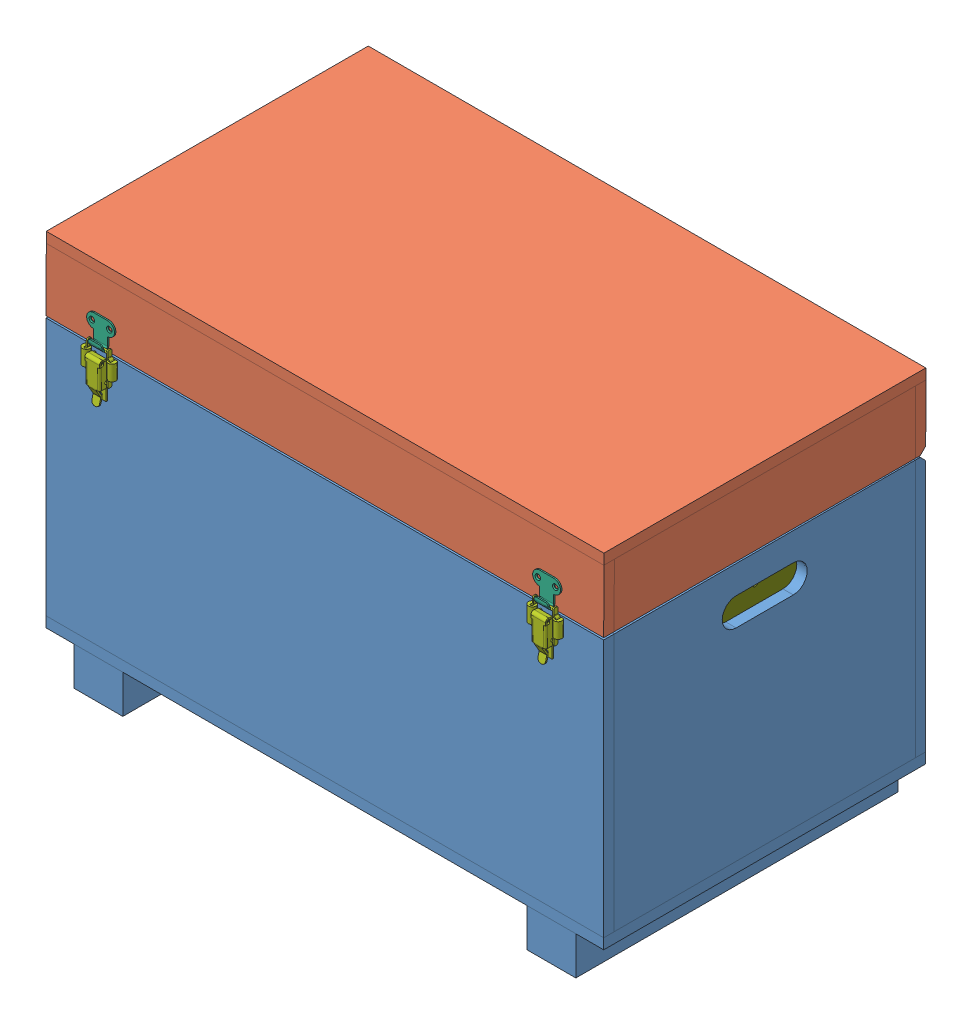
SolidWorks assembly 2021_CaisseTransport, configuration Default. Lengths in mm.
Overall size (800 575.29 476.19).
36 component instances, 27 part files, 81 mates.
Components (placement in the parent):
- 2021_Caisse_Fond-1: 2021_Caisse_Fond [Default] at origin size (800 446 462)
- 2021_Caisse_Capot-1: 2021_Caisse_Capot [Default] at (0 492.3908 -0.1871) x (-1 0 0) z (0 0.001745 0.999998) size (800 124 462)
- _2021_RobotPrincipal_FacesExt-1: _2021_RobotPrincipal_FacesExt [Default] at (-195 34.5 15) x (0 0 -1) z (1 0 0) size (333 431 295.5)
- _2021_RobotSecondaire_FacesExt-1: _2021_RobotSecondaire_FacesExt [Default] at (72 34.5 -65) x (-1 0 0) z (0 0 -1) size (273 428.5 191)
- _2021_Phare_FacesExt-1: _2021_Phare_FacesExt [Default] at (146 145 117) x (-1 0 0) z (0 0 -1) size (440.05 342.73 212.15)
- carton_clavier_logitech_k400-1: carton_clavier_logitech_k400 [Défaut] at (-278.5 201 -214) x (0 -1 0) z (-1 0 0) size (372 32 155)
- Plateau roulant Manutention-1: Plateau roulant Manutention [Défaut] x (-1 0 0) z (0 0 -1) size (575 82.5 290)
- StationAccueil-1: StationAccueil [Défaut] at (17 215 -192) x (0 1 0) z (1 0 0) size (428 34 400)
- GL-210606-0849_CaissePce01-1: GL-210606-0849_CaissePce01 [Default] at (-192 215 -216) size (43.02 40.06 45)
- GL-210606-0853_CaissePce02-1: GL-210606-0853_CaissePce02 [Default] at (-364 210 -216) size (26.02 40.06 45)
- GL-210606-0904_CaissePce03-1: GL-210606-0904_CaissePce03 [Default] at (217 210 -151) x (-1 0 0) z (0 0 -1) size (16.03 40.06 30)
- GL-210606-0912_CaissePce04-1: GL-210606-0912_CaissePce04 [Default] at (-385 374 147) size (10.79 44 25.48)
- GL-210606-0912_CaissePce04-2: GL-210606-0912_CaissePce04 [Default] at (385 374 147) x (-1 0 0) z (0 0 -1) size (10.79 44 25.48)
- GL-210606-0912_CaissePce04-3: GL-210606-0912_CaissePce04 [Default] at (-78 134 189) x (-1 0 0) z (0 0 -1) size (10.79 44 25.48)
- GL-210606-0943_CaissePce05-1: GL-210606-0943_CaissePce05 [Default] at (-56.5 15 -118.5) size (45.57 49.43 53.44)
- GL-210606-0943_CaissePce05-2: GL-210606-0943_CaissePce05 [Default] at (200.5 15 -11.5) x (-1 0 0) z (0 0 -1) size (45.57 49.43 53.44)
- GL-210606-0943_CaissePce05_Sym-3: GL-210606-0943_CaissePce05_Sym [Default] at (-56.5 15 -11.5) size (45.57 49.43 53.44)
- GL-210606-0943_CaissePce05_Sym-4: GL-210606-0943_CaissePce05_Sym [Default] at (200.5 15 -118.5) x (-1 0 0) z (0 0 -1) size (45.57 49.43 53.44)
- GL-210606-1029_CaissePce06-1: GL-210606-1029_CaissePce06 [Default] at (-141.5 15 -143.5) x (0 0 1) z (-1 0 0) size (35.58 49.93 35.5)
- _2021_VisionCentrale_FacesExt-1: _2021_VisionCentrale_FacesExt [Default] at (275.4 230 -111) x (0 1 0) z (0 0 1) size (244.44 54.3 190)
- GL-210606-1436_CaissePce07-2: GL-210606-1436_CaissePce07 [Default] at (-248.5 15 173.5) x (0 0 -1) z (1 0 0) size (35.58 49.43 55.65)
- GL-210606-1436_CaissePce07_Sym-2: GL-210606-1436_CaissePce07_Sym [Default] at (-248.5 15 -143.5) x (0 0 1) z (-1 0 0) size (35.58 49.43 55.65)
- GL-210606-1029_CaissePce06_Sym-2: GL-210606-1029_CaissePce06_Sym [Default] at (-141.5 15 173.5) x (0 0 -1) z (1 0 0) size (35.58 49.93 35.5)
- GL-210606-1457_CaissePce08-1: GL-210606-1457_CaissePce08 [Default] at (-346 15 15) size (27.07 49.43 30)
- GL-210606-1507_CaissePce09-2: GL-210606-1507_CaissePce09 [Default] at (235 132 -7) x (0 0 -1) z (1 0 0) size (32 160 63.05)
- GL-210606-1507_CaissePce09_Sym-3: GL-210606-1507_CaissePce09_Sym [Default] at (235 132 -215) x (0 0 1) z (-1 0 0) size (32 160 63.05)
- GL-210606-1534_CaissePce10-1: GL-210606-1534_CaissePce10 [Default] at (-342.5 330 216) x (0 0 -1) z (0 -1 0) size (30.57 15 56.89)
- GL-210606-1534_CaissePce10-2: GL-210606-1534_CaissePce10 [Default] at (-297.5 330 216) x (0 0 -1) z (0 -1 0) size (30.57 15 56.89)
- FermoirRessort_PartB-1: FermoirRessort_PartB [Default] at (-320 417.7941 230.9435) x (1 0 0) z (0 0.001745 0.999998) size (40 37 10)
- FermoirRessort_PartA-1: FermoirRessort_PartA [Default] at (-320 360 231) size (48 75.52 15.5)
- FermoirRessort_PartA-2: FermoirRessort_PartA [Default] at (320 360 231) size (48 75.52 15.5)
- FermoirRessort_PartB-2: FermoirRessort_PartB [Default] at (320 417.7941 230.9435) x (1 0 0) z (0 0.001745 0.999998) size (40 37 10)
- GL-210607-2320_CaissePce11-1: GL-210607-2320_CaissePce11 [Default] at (-195 470.6875 169.851) x (1 0 0) z (0 -0.001745 -0.999998) size (190 80 29)
- GL-210607-2320_CaissePce11-2: GL-210607-2320_CaissePce11 [Default] at (-195 470.1465 -140.1485) x (1 0 0) z (0 -0.001745 -0.999998) size (190 80 29)
- GL-210607-2322_CaissePce12-1: GL-210607-2322_CaissePce12 [Default] at (-53 470.2774 -65.1486) x (0 0.001745 0.999998) z (1 0 0) size (220 80 29)
- GL-210607-2322_CaissePce12-2: GL-210607-2322_CaissePce12 [Default] at (197 470.2774 -65.1486) x (0 0.001745 0.999998) z (1 0 0) size (220 80 29)
Mates (geometry in assembly coordinates):
- Coïncidente1: coincident: circle of assembly; circle of assembly; circle of 2021_Caisse_Fond-1; circle of 2021_Caisse_Capot-1
- AngleLimite1: limit planar angle = 0.001745 rad: plane of assembly; plane of assembly; plane of 2021_Caisse_Capot-1 through (0 387.391 -0.0038) normal (0 -0.999998 0.001745); plane of 2021_Caisse_Fond-1 through (0 385 0) normal (0 1 0)
- Distance12: distance = 25 mm: plane of assembly; plane of assembly; plane of _2021_RobotSecondaire_FacesExt-1 through (72 40 -105) normal (0 -1 0); plane of 2021_Caisse_Fond-1 through (0 15 0) normal (0 1 0)
- Distance13: distance = 25 mm: plane of _2021_RobotPrincipal_FacesExt-1 through (-195 40 15) normal (0 -1 0); plane of 2021_Caisse_Fond-1 through (0 15 0) normal (0 1 0)
- Coïncidente26: coincident: plane of assembly; plane of assembly; plane of 2021_Caisse_Fond-1 through (0 15 0) normal (0 1 0); plane of StationAccueil-1 through (217 15 -214) normal (0 -1 0)
- Coïncidente13: coincident: plane of assembly; plane of assembly; plane of 2021_Caisse_Fond-1 through (0 0 0) normal (0 -1 0); plane of Plateau roulant Manutention-1 through (0 0 0) normal (0 1 0)
- Coïncidente14: coincident: plane of assembly through (0 0 0) normal (0 0 1); plane of Plateau roulant Manutention-1 through (0 0 0) normal (0 0 -1); plane of assembly
- Coïncidente15: coincident: plane of assembly through (0 0 0) normal (1 0 0); plane of Plateau roulant Manutention-1 through (0 0 0) normal (-1 0 0); plane of assembly
- Distance19: distance = 72 mm: plane of assembly through (0 0 0) normal (1 0 0); plane of assembly; plane of _2021_RobotSecondaire_FacesExt-1 through (72 34.5 -65) normal (-1 0 0)
- Distance6: distance = 65 mm: plane of assembly through (0 0 0) normal (0 0 1); plane of _2021_RobotSecondaire_FacesExt-1 through (72 34.5 -65) normal (0 0 -1); plane of assembly
- Distance7: distance = 195 mm: plane of _2021_RobotPrincipal_FacesExt-1 through (-195 34.5 15) normal (1 0 0); plane of assembly through (0 0 0) normal (1 0 0)
- Distance14: distance = 15 mm: plane of _2021_RobotPrincipal_FacesExt-1 through (-195 34.5 15) normal (0 0 -1); plane of assembly through (0 0 0) normal (0 0 1)
- Distance11: distance = 130 mm: plane of assembly; plane of assembly; plane of _2021_Phare_FacesExt-1 through (146 145 117) normal (0 -1 0); plane of 2021_Caisse_Fond-1 through (0 15 0) normal (0 1 0)
- Distance15: distance = 1 mm: plane of StationAccueil-1 through (17 215 -215) normal (0 0 -1); plane of 2021_Caisse_Fond-1 through (-400 385 -216) normal (0 0 1)
- Distance16: distance = 2 mm: plane of assembly; plane of assembly; plane of carton_clavier_logitech_k400-1 through (-278.5 201 -214) normal (0 0 -1); plane of 2021_Caisse_Fond-1 through (-400 385 -216) normal (0 0 1)
- Coïncidente29: coincident: plane of 2021_Caisse_Fond-1 through (0 15 0) normal (0 1 0); plane of carton_clavier_logitech_k400-1 through (-356 15 -182) normal (0 -1 0)
- Distance17: distance = 4 mm: plane of _2021_Phare_FacesExt-1 through (366 373.5 145) normal (1 0 0); plane of 2021_Caisse_Fond-1 through (370 434.3356 216) normal (-1 0 0)
- Distance18: distance = 4 mm: plane of _2021_Phare_FacesExt-1 through (366 146.5 212) normal (0 0 1); plane of 2021_Caisse_Fond-1 through (-400 385 216) normal (0 0 -1)
- Distance20: distance = 3 mm: plane of StationAccueil-1 through (217 415 -214) normal (1 0 0); plane of 2021_Caisse_Fond-1 through (220 527.429 -216) normal (-1 0 0)
- Distance21: distance = 18 mm: plane of StationAccueil-1 through (-183 15 -214) normal (-1 0 0); plane of carton_clavier_logitech_k400-1 through (-201 387 -182) normal (1 0 0)
- Coïncidente30: coincident: plane of assembly; plane of assembly; plane of 2021_Caisse_Fond-1 through (-400 385 -216) normal (0 0 1); plane of GL-210606-0849_CaissePce01-1 through (-199.5 235 -216) normal (0 0 -1)
- Distance22: distance = 9 mm: plane of GL-210606-0849_CaissePce01-1 through (-192 215 -216) normal (1 0 0); plane of StationAccueil-1 through (-183 15 -214) normal (-1 0 0)
- Distance23: distance = 220 mm: plane of GL-210606-0849_CaissePce01-1 through (-192 235 -216) normal (0 1 0); plane of 2021_Caisse_Fond-1 through (0 15 0) normal (0 1 0)
- Coïncidente33: coincident: plane of GL-210606-0849_CaissePce01-1 through (-192 235 -216) normal (0 1 0); plane of GL-210606-0853_CaissePce02-1 through (-364 235 -216) normal (0 1 0)
- Coïncidente34: coincident: plane of 2021_Caisse_Fond-1 through (-370 434.3356 -216) normal (1 0 0); plane of GL-210606-0853_CaissePce02-1 through (-370 195 -171) normal (-1 0 0)
- Coïncidente35: coincident: plane of 2021_Caisse_Fond-1 through (-400 385 -216) normal (0 0 1); plane of GL-210606-0853_CaissePce02-1 through (-370 195 -216) normal (0 0 -1)
- Coïncidente36: coincident: plane of GL-210606-0849_CaissePce01-1 through (-192 235 -216) normal (0 1 0); plane of GL-210606-0904_CaissePce03-1 through (217 235 -151) normal (0 1 0)
- Coïncidente37: coincident: plane of GL-210606-0849_CaissePce01-1 through (-184.5 235 -181) normal (0 0 -1); plane of GL-210606-0904_CaissePce03-1 through (204 195 -181) normal (0 0 -1)
- Coïncidente38: coincident: plane of 2021_Caisse_Fond-1 through (220 527.429 -216) normal (-1 0 0); plane of GL-210606-0904_CaissePce03-1 through (220 195 -181) normal (1 0 0)
- Distance28: distance = 15 mm: plane of assembly; plane of assembly; plane of 2021_Caisse_Fond-1 through (-400 385 216) normal (0 0 -1); plane of GL-210606-0912_CaissePce04-3 through (-78 120 201) normal (0 0 1)
- Coïncidente40: coincident: plane of 2021_Caisse_Fond-1 through (-78 145 216) normal (-1 0 0); plane of GL-210606-0912_CaissePce04-3 through (-78 120 177) normal (1 0 0)
- Coïncidente41: coincident: plane of assembly; plane of assembly; plane of GL-210606-0912_CaissePce04-1 through (-375 360 159) normal (0 0 1); plane of GL-210606-0912_CaissePce04-2 through (385 360 159) normal (0 0 1)
- Coïncidente42: coincident: plane of GL-210606-0912_CaissePce04-1 through (-385 404 147) normal (0 1 0); plane of GL-210606-0912_CaissePce04-2 through (385 404 147) normal (0 1 0)
- Coïncidente43: coincident: plane of 2021_Caisse_Fond-1 through (-385 385 -216) normal (1 0 0); plane of GL-210606-0912_CaissePce04-1 through (-385 360 159) normal (-1 0 0)
- Coïncidente44: coincident: plane of 2021_Caisse_Fond-1 through (385 385 -216) normal (-1 0 0); plane of GL-210606-0912_CaissePce04-2 through (385 360 135) normal (1 0 0)
- Distance24: distance = 10 mm: plane of GL-210606-0912_CaissePce04-2 through (385 360 159) normal (0 0 1); plane of 2021_Caisse_Fond-1 through (385 434.3356 169) normal (0 0 -1)
- Distance26: distance = 25 mm: plane of GL-210606-0912_CaissePce04-1 through (-385 360 147) normal (0 -1 0); plane of 2021_Caisse_Fond-1 through (0 385 0) normal (0 1 0)
- Distance27: distance = 25 mm: plane of GL-210606-0912_CaissePce04-3 through (-78 120 189) normal (0 -1 0); plane of 2021_Caisse_Fond-1 through (0 145 0) normal (0 1 0)
- Coïncidente49: coincident: plane of assembly; plane of assembly; plane of 2021_Caisse_Fond-1 through (0 15 0) normal (0 1 0); plane of GL-210606-0943_CaissePce05-1 through (-56.5 15 -118.5) normal (0 -1 0)
- Coaxiale1: concentric: point of assembly; cylinder of assembly; point of GL-210606-0943_CaissePce05-1; cylinder of _2021_RobotSecondaire_FacesExt-1 through (-56.5 50.25 -118.5) axis (0 -1 0) radius 8
- Parallèle2: parallel: plane of assembly; plane of assembly; plane of _2021_RobotSecondaire_FacesExt-1 through (72 45.5 -5) normal (0 0 1); plane of GL-210606-0943_CaissePce05-1 through (-56.5 15 -118.5) normal (0 0 1)
- Coïncidente53: coincident: plane of assembly; plane of assembly; plane of GL-210606-0943_CaissePce05-1 through (-56.5 15 -118.5) normal (0 -1 0); plane of GL-210606-0943_CaissePce05-2 through (200.5 15 -11.5) normal (0 -1 0)
- Parallèle3: parallel: plane of assembly; plane of assembly; plane of GL-210606-0943_CaissePce05-1 through (-64 40 -102.5) normal (0 0 1); plane of GL-210606-0943_CaissePce05-2 through (208 40 -27.5) normal (0 0 -1)
- Coaxiale2: concentric: cylinder of assembly; point of assembly; cylinder of _2021_RobotSecondaire_FacesExt-1 through (200.5 50.25 -11.5) axis (0 -1 0) radius 8; point of GL-210606-0943_CaissePce05-2
- Coïncidente56: coincident: plane of 2021_Caisse_Fond-1 through (0 15 0) normal (0 1 0); plane of GL-210606-1029_CaissePce06-1 through (-141.5 15 -143.5) normal (0 -1 0)
- Coaxiale3: concentric: cylinder of _2021_RobotPrincipal_FacesExt-1 through (-141.5 50.25 -143.5) axis (0 -1 0) radius 8; unknown of GL-210606-1029_CaissePce06-1
- Parallèle4: parallel: plane of _2021_RobotPrincipal_FacesExt-1 through (-135 45.5 15) normal (1 0 0); plane of GL-210606-1029_CaissePce06-1 through (-141.5 15 -143.5) normal (-1 0 0)
- Distance29: distance = 8 mm: plane of _2021_VisionCentrale_FacesExt-1 through (243 315 -206) normal (-1 0 0); plane of 2021_Caisse_Fond-1 through (235 527.429 -216) normal (1 0 0)
- Distance30: distance = 10 mm: plane of _2021_VisionCentrale_FacesExt-1 through (247.1 135 -206) normal (0 0 -1); plane of 2021_Caisse_Fond-1 through (-400 385 -216) normal (0 0 1)
- Distance31: distance = 120 mm: plane of _2021_VisionCentrale_FacesExt-1 through (247.1 135 -206) normal (0 -1 0); plane of 2021_Caisse_Fond-1 through (0 15 0) normal (0 1 0)
- Coïncidente57: coincident: plane of 2021_Caisse_Fond-1 through (0 15 0) normal (0 1 0); plane of GL-210606-1436_CaissePce07-2 through (-195 15 15) normal (0 -1 0)
- Coaxiale4: concentric: cylinder of _2021_RobotPrincipal_FacesExt-1 through (-248.5 50.25 173.5) axis (0 -1 0) radius 8; unknown of GL-210606-1436_CaissePce07-2
- Parallèle5: parallel: plane of _2021_RobotPrincipal_FacesExt-1 through (-255 45.5 180) normal (0 0 1); plane of GL-210606-1436_CaissePce07-2 through (-248.5 15 173.5) normal (0 0 -1)
- Coïncidente60: coincident: plane of assembly; plane of assembly; plane of 2021_Caisse_Fond-1 through (0 15 0) normal (0 1 0); plane of GL-210606-1457_CaissePce08-1 through (-346 15 15) normal (0 -1 0)
- Distance32: distance = 1 mm: plane of GL-210606-1457_CaissePce08-1 through (-346 -17.311 0) normal (1 0 0); plane of _2021_RobotPrincipal_FacesExt-1 through (-345 41.5 -73.1816) normal (-1 0 0)
- Coïncidente62: coincident: plane of _2021_RobotPrincipal_FacesExt-1 through (-195 34.5 15) normal (0 0 -1); plane of GL-210606-1457_CaissePce08-1 through (-346 15 15) normal (0 0 1)
- Coïncidente63: coincident: plane of 2021_Caisse_Fond-1 through (235 527.429 -216) normal (1 0 0); plane of GL-210606-1507_CaissePce09-2 through (235 292 -26) normal (-1 0 0)
- Coïncidente64: coincident: plane of 2021_Caisse_Fond-1 through (0 265 0) normal (0 1 0); plane of GL-210606-1507_CaissePce09-2 through (235 265 -22) normal (0 -1 0)
- Distance33: distance = 2 mm: plane of GL-210606-1507_CaissePce09-2 through (242 292 -14) normal (0 0 -1); plane of _2021_VisionCentrale_FacesExt-1 through (247.1 135 -16) normal (0 0 1)
- Coïncidente66: coincident: plane of assembly; plane of assembly; plane of 2021_Caisse_Fond-1 through (-400 385 216) normal (0 0 -1); plane of GL-210606-1534_CaissePce10-1 through (-335 350 216) normal (0 0 1)
- Distance34: distance = 20 mm: plane of GL-210606-1534_CaissePce10-1 through (-350 352.8914 203.4271) normal (-1 0 0); plane of 2021_Caisse_Fond-1 through (-370 434.3356 216) normal (1 0 0)
- Distance35: distance = 35 mm: plane of GL-210606-1534_CaissePce10-1 through (-335 350 213) normal (0 1 0); plane of 2021_Caisse_Fond-1 through (0 385 0) normal (0 1 0)
- Coïncidente69: coincident: plane of GL-210606-1534_CaissePce10-1 through (-335 350 216) normal (0 0 1); plane of GL-210606-1534_CaissePce10-2 through (-290 350 216) normal (0 0 1)
- Coïncidente70: coincident: plane of GL-210606-1534_CaissePce10-1 through (-335 350 213) normal (0 1 0); plane of GL-210606-1534_CaissePce10-2 through (-290 350 213) normal (0 1 0)
- Distance36: distance = 30 mm: plane of GL-210606-1534_CaissePce10-1 through (-335 352.8914 203.4271) normal (1 0 0); plane of GL-210606-1534_CaissePce10-2 through (-305 352.8914 203.4271) normal (-1 0 0)
- Coïncidente72: coincident: plane of assembly; plane of assembly; plane of 2021_Caisse_Capot-1 through (400 387.7941 230.9958) normal (0 0.001745 0.999998); plane of FermoirRessort_PartB-1 through (-310 427.7941 230.926) normal (0 -0.001745 -0.999998)
- Distance37: distance = 80 mm: plane of assembly; plane of assembly; plane of FermoirRessort_PartB-1 through (-320 417.7941 230.9435) normal (1 0 0); plane of 2021_Caisse_Capot-1 through (-400 387.014 -216.0035) normal (-1 0 0)
- Distance38: distance = 30 mm: plane of assembly; plane of assembly; plane of FermoirRessort_PartB-1 through (-320 417.7941 230.9435) normal (0 0.999998 -0.001745); plane of 2021_Caisse_Capot-1 through (0 387.391 -0.0038) normal (0 -0.999998 0.001745)
- Coïncidente75: coincident: plane of assembly; plane of assembly; plane of 2021_Caisse_Fond-1 through (-400 385 231) normal (0 0 1); plane of FermoirRessort_PartA-1 through (-312 326 231) normal (0 0 -1)
- Coïncidente76: coincident: plane of assembly; plane of assembly; plane of FermoirRessort_PartB-1 through (-320 417.7941 230.9435) normal (1 0 0); plane of FermoirRessort_PartA-1 through (-320 360 231) normal (1 0 0)
- Distance39: distance = 25 mm: plane of assembly; plane of assembly; plane of FermoirRessort_PartA-1 through (-320 360 231) normal (0 1 0); plane of 2021_Caisse_Fond-1 through (0 385 0) normal (0 1 0)
- Coïncidente77: coincident: plane of assembly; plane of assembly; plane of GL-210607-2322_CaissePce12-1 through (-38.5 470.1203 -155.1485) normal (0 -0.202984 -0.979182); plane of GL-210607-2322_CaissePce12-2 through (211.5 470.1203 -155.1485) normal (0 -0.202984 -0.979182)
- Coïncidente78: coincident: plane of GL-210607-2322_CaissePce12-1 through (-38.5 397.1466 -140.0211) normal (0 -0.999998 0.001745); plane of GL-210607-2322_CaissePce12-2 through (211.5 397.1466 -140.0211) normal (0 -0.999998 0.001745)
- Coïncidente79: coincident: plane of assembly; plane of assembly; plane of GL-210607-2320_CaissePce11-1 through (-120 470.6622 155.3511) normal (0.979535 -0.201274 0.000351); plane of GL-210607-2320_CaissePce11-2 through (-120 470.1212 -154.6485) normal (0.979535 -0.201274 0.000351)
- Coïncidente80: coincident: plane of GL-210607-2320_CaissePce11-1 through (-135 397.6623 155.4785) normal (0 -0.999998 0.001745); plane of GL-210607-2320_CaissePce11-2 through (-135 397.1213 -154.521) normal (0 -0.999998 0.001745)
- Coïncidente81: coincident: plane of 2021_Caisse_Capot-1 through (0 477.3908 -0.1609) normal (0 -0.999998 0.001745); plane of GL-210607-2320_CaissePce11-1 through (-100 477.6622 155.3389) normal (0 0.999998 -0.001745)
- Coïncidente82: coincident: plane of 2021_Caisse_Capot-1 through (0 477.3908 -0.1609) normal (0 -0.999998 0.001745); plane of GL-210607-2322_CaissePce12-1 through (-38.5 477.0854 -175.1606) normal (0 0.999998 -0.001745)
- Coïncidente83: coincident: line of 2021_Caisse_Capot-1 through (-255 368.713 184.529) axis (0 0.999998 -0.001745); unknown of GL-210607-2320_CaissePce11-1
- Coïncidente84: coincident: point of 2021_Caisse_Capot-1; point of GL-210607-2320_CaissePce11-2
- Coïncidente85: coincident: point of 2021_Caisse_Capot-1; point of GL-210607-2322_CaissePce12-1
- Coïncidente86: coincident: point of 2021_Caisse_Capot-1; point of GL-210607-2322_CaissePce12-2
